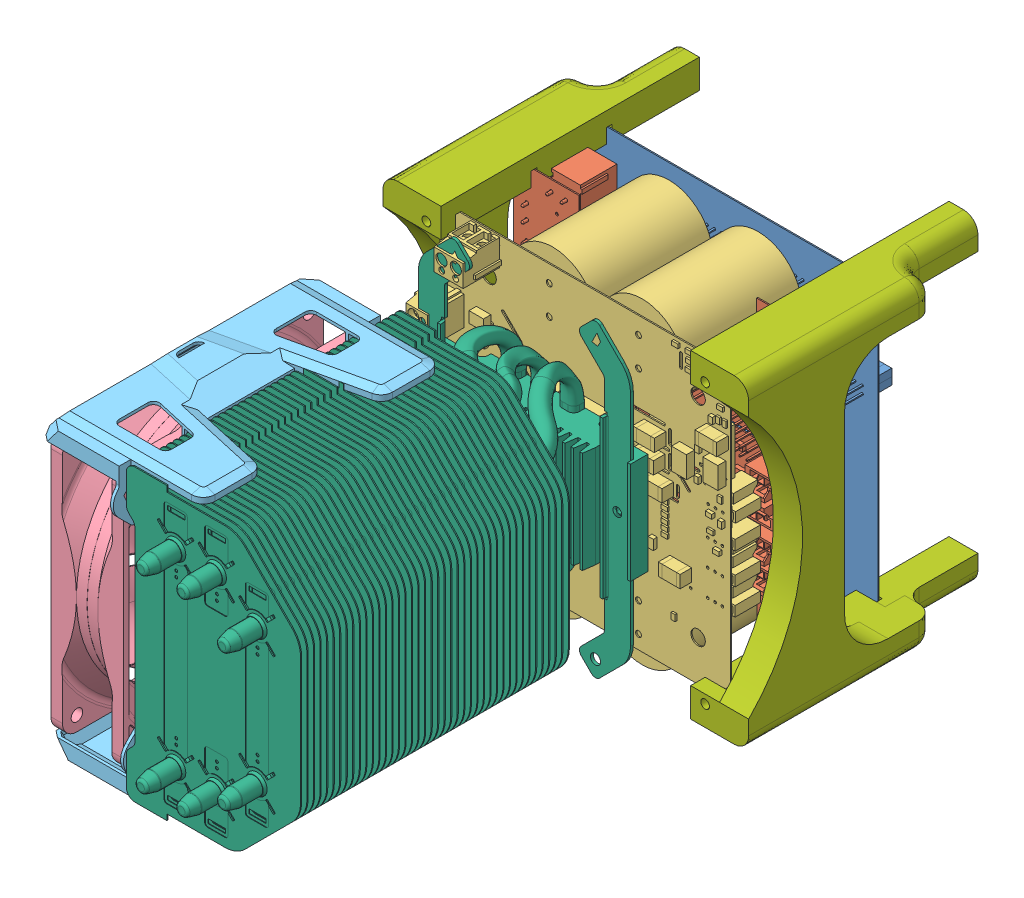
SolidWorks assembly REV3.0, configuration Default. Lengths in mm.
Overall size (190.84 111.69 228.07).
10 component instances, 7 part files, 14 mates.
Components (placement in the parent):
- controlo_rev3-1: controlo_rev3 [Default] at (-50.1858 -26.7845 -12.6892) size (100.07 100.84 29.54)
- middlePCB_rev3-1: middlePCB_rev3 [Default] at (-50.1858 -26.7845 12.7222) size (100.36 100.9 32.46)
- inversor_rev3-1: inversor_rev3 [Default] at (-50.1858 -26.7845 38.1337) size (100.35 109.25 56.47)
- dissipador-1: dissipador [Default] at (4.979 -21.2139 126.7824) x (0 1 0) z (0 0 1) size (108.44 180.01 139.76)
  - 7030025_PART_FAN STANDARD 90_MODEL.igs-1: 7030025_PART_FAN STANDARD 90_MODEL.igs [Default] at (0 45 -45) x (1 0 0) z (0 -1 0) size (93.98 180.01 25.07)
  - 7030026_PART_HEATSINK ADAPTOR 90_MODEL.igs-1: 7030026_PART_HEATSINK ADAPTOR 90_MODEL.igs [Default] at (95 58.5 47.4641) x (0 0 -1) z (-1 0 0) size (106.39 52.6 26.58)
  - 7030026_PART_HEATSINK ADAPTOR 90_MODEL.igs-2: 7030026_PART_HEATSINK ADAPTOR 90_MODEL.igs [Default] at (-7 58.5 -46) x (0 0 1) z (1 0 0) size (106.39 52.6 26.58)
  - 7030027_PART_CPU HEATSINK TOWER_MODEL.igs-1: 7030027_PART_CPU HEATSINK TOWER_MODEL.igs [Default] at (94 31.5 -47.65) x (-1 0 0) z (0 0 1) size (108.44 80.01 139.76)
- suporte_conversor_rev31-1: suporte_conversor_rev31 [Default] at (-45.1858 21.2155 12.7222) x (0 -1 0) z (-1 0 0) size (110 89 20)
- suporte_conversor_rev31-2: suporte_conversor_rev31 [Default] at (40.8142 21.2155 12.7222) x (0 1 0) z (1 0 0) size (110 89 20)
Mates (geometry in assembly coordinates):
- Concentric1: concentric: cylinder of middlePCB_rev3-1 through (-50.1858 69.2155 12.3108) axis (0 0 -1) radius 1.5; cylinder of inversor_rev3-1 through (-50.1858 69.2155 37.7222) axis (0 0 -1) radius 1.5
- Concentric2: concentric: cylinder of controlo_rev3-1 through (-50.1858 69.2155 -13.1007) axis (0 0 -1) radius 1.5; cylinder of middlePCB_rev3-1 through (-50.1858 69.2155 12.3108) axis (0 0 -1) radius 1.5
- Concentric3: concentric: cylinder of middlePCB_rev3-1 through (45.8142 69.2155 12.3108) axis (0 0 -1) radius 1.5; cylinder of inversor_rev3-1 through (45.8142 69.2155 37.7222) axis (0 0 -1) radius 1.5
- Concentric4: concentric: cylinder of controlo_rev3-1 through (45.8142 69.2155 -13.1007) axis (0 0 -1) radius 1.5; cylinder of middlePCB_rev3-1 through (45.8142 69.2155 12.3108) axis (0 0 -1) radius 1.5
- Distance1: distance = 25 mm: plane of middlePCB_rev3-1 through (-52.0908 -28.7895 12.7222) normal (0 0 1); plane of inversor_rev3-1 through (-52.1858 -28.6895 37.7222) normal (0 0 -1)
- Distance2: distance = 25 mm: plane of middlePCB_rev3-1 through (-52.0908 -28.7895 12.3108) normal (0 0 -1); plane of controlo_rev3-1 through (-52.1858 -28.6895 -12.6892) normal (0 0 1)
- Tangent2: tangent: plane of inversor_rev3-1 through (-3.8278 39.0361 44.1324) normal (0 0 1); face of dissipador-1/7030027_PART_CPU HEATSINK TOWER_MODEL.igs-1
- Tangent5: tangent: plane of inversor_rev3-1 through (-2.0778 40.2861 44.1324) normal (0 1 0); face of dissipador-1/7030027_PART_CPU HEATSINK TOWER_MODEL.igs-1
- Concentric5: concentric: cylinder of inversor_rev3-1 through (-50.1858 69.2155 37.7222) axis (0 0 -1) radius 1.5; cylinder of suporte_conversor_rev31-1 through (-50.1858 69.2155 -12.2778) axis (0 0 1) radius 1.5
- Concentric6: concentric: cylinder of inversor_rev3-1 through (-50.1858 -26.7845 37.7222) axis (0 0 -1) radius 1.5; cylinder of suporte_conversor_rev31-1 through (-50.1858 -26.7845 48.9649) axis (0 0 -1) radius 1.5
- Coincident1: coincident: plane of inversor_rev3-1 through (-52.1858 -28.6895 37.7222) normal (0 0 -1); plane of suporte_conversor_rev31-1 through (-55.1858 21.2155 37.7222) normal (0 0 1)
- Coincident2: coincident: cylinder of inversor_rev3-1 through (45.8142 -26.7845 37.7222) axis (0 0 -1) radius 1.5; circle of suporte_conversor_rev31-2
- Coincident3: coincident: plane of inversor_rev3-1 through (-52.1858 -28.6895 37.7222) normal (0 0 -1); plane of suporte_conversor_rev31-2 through (50.8142 21.2155 37.7222) normal (0 0 1)
- Concentric7: concentric: cylinder of inversor_rev3-1 through (45.8142 69.2155 37.7222) axis (0 0 -1) radius 1.5; cylinder of suporte_conversor_rev31-2 through (45.8142 69.2155 48.9649) axis (0 0 -1) radius 1.5
